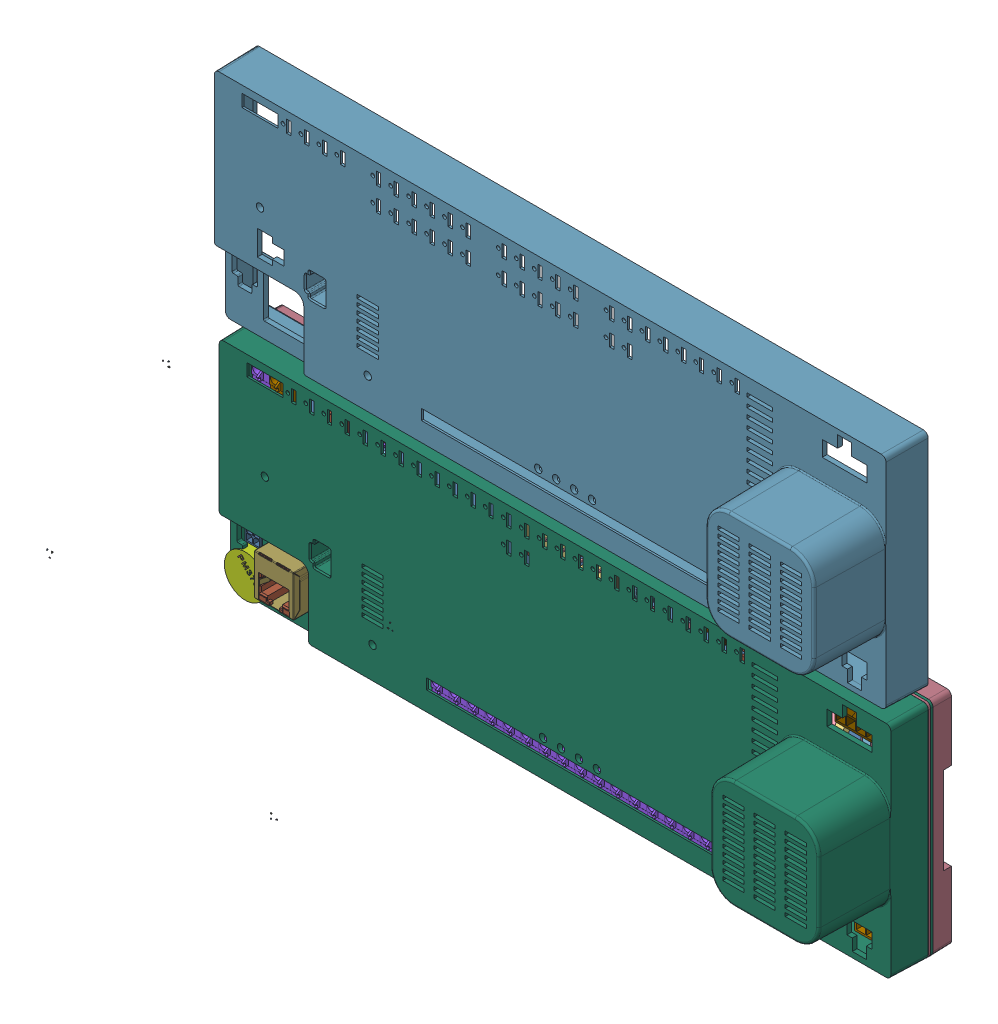
SolidWorks assembly _SC944D, configuration Default. Lengths in mm. (continued)
Components (placement in the parent): (continued)
- U10-1: U10 [Default] at origin size (22 22 1.6) (continued)
  - User_Library-LQFP144-1: User_Library-LQFP144 [Default] at (60.232 23.8429 0) x (-1 0 0) z (0 1 0) size (22 1.6 22) (continued)
    - User_Library-LQFP144_Assu_Fuss_LQFP144-4: User_Library-LQFP144_Assu_Fuss_LQFP144 [Default] at (-10 0 0) x (-1 0 0) z (0 0 -1) size (1 0.89 17.72) (continued)
      - User_Library-LQFP144_Fuss_LQFP144-3: User_Library-LQFP144_Fuss_LQFP144 [Default] at (0 0 -3.75) size (1 0.89 0.22)
      - User_Library-LQFP144_Fuss_LQFP144-4: User_Library-LQFP144_Fuss_LQFP144 [Default] at (0 0 -0.25) size (1 0.89 0.22)
      - User_Library-LQFP144_Fuss_LQFP144-5: User_Library-LQFP144_Fuss_LQFP144 [Default] at (0 0 -5.25) size (1 0.89 0.22)
      - User_Library-LQFP144_Fuss_LQFP144-6: User_Library-LQFP144_Fuss_LQFP144 [Default] at (0 0 -8.25) size (1 0.89 0.22)
      - User_Library-LQFP144_Fuss_LQFP144-7: User_Library-LQFP144_Fuss_LQFP144 [Default] at (0 0 -0.25) size (1 0.89 0.22)
      - User_Library-LQFP144_Fuss_LQFP144-8: User_Library-LQFP144_Fuss_LQFP144 [Default] at (0 0 -3.75) size (1 0.89 0.22)
      - User_Library-LQFP144_Fuss_LQFP144-9: User_Library-LQFP144_Fuss_LQFP144 [Default] at (0 0 -0.25) size (1 0.89 0.22)
      - User_Library-LQFP144_Fuss_LQFP144-10: User_Library-LQFP144_Fuss_LQFP144 [Default] at (0 0 6.75) size (1 0.89 0.22)
      - User_Library-LQFP144_Fuss_LQFP144-11: User_Library-LQFP144_Fuss_LQFP144 [Default] at (0 0 -3.75) size (1 0.89 0.22)
      - User_Library-LQFP144_Fuss_LQFP144-12: User_Library-LQFP144_Fuss_LQFP144 [Default] at (0 0 4.25) size (1 0.89 0.22)
      - User_Library-LQFP144_Fuss_LQFP144-13: User_Library-LQFP144_Fuss_LQFP144 [Default] at (0 0 0.75) size (1 0.89 0.22)
      - User_Library-LQFP144_Fuss_LQFP144-14: User_Library-LQFP144_Fuss_LQFP144 [Default] at (0 0 7.75) size (1 0.89 0.22)
      - User_Library-LQFP144_Fuss_LQFP144-15: User_Library-LQFP144_Fuss_LQFP144 [Default] at (0 0 1.75) size (1 0.89 0.22)
      - User_Library-LQFP144_Fuss_LQFP144-16: User_Library-LQFP144_Fuss_LQFP144 [Default] at (0 0 -2.25) size (1 0.89 0.22)
      - User_Library-LQFP144_Fuss_LQFP144-17: User_Library-LQFP144_Fuss_LQFP144 [Default] at (0 0 -2.75) size (1 0.89 0.22)
      - User_Library-LQFP144_Fuss_LQFP144-18: User_Library-LQFP144_Fuss_LQFP144 [Default] at (0 0 -4.25) size (1 0.89 0.22)
      - User_Library-LQFP144_Fuss_LQFP144-19: User_Library-LQFP144_Fuss_LQFP144 [Default] at (0 0 3.25) size (1 0.89 0.22)
      - User_Library-LQFP144_Fuss_LQFP144-20: User_Library-LQFP144_Fuss_LQFP144 [Default] at (0 0 -1.75) size (1 0.89 0.22)
      - User_Library-LQFP144_Fuss_LQFP144-21: User_Library-LQFP144_Fuss_LQFP144 [Default] at (0 0 -1.75) size (1 0.89 0.22)
      - User_Library-LQFP144_Fuss_LQFP144-22: User_Library-LQFP144_Fuss_LQFP144 [Default] at (0 0 2.75) size (1 0.89 0.22)
      - User_Library-LQFP144_Fuss_LQFP144-23: User_Library-LQFP144_Fuss_LQFP144 [Default] at (0 0 -2.75) size (1 0.89 0.22)
      - User_Library-LQFP144_Fuss_LQFP144-24: User_Library-LQFP144_Fuss_LQFP144 [Default] at (0 0 -3.75) size (1 0.89 0.22)
      - User_Library-LQFP144_Fuss_LQFP144-25: User_Library-LQFP144_Fuss_LQFP144 [Default] at (0 0 -5.75) size (1 0.89 0.22)
      - User_Library-LQFP144_Fuss_LQFP144-26: User_Library-LQFP144_Fuss_LQFP144 [Default] at (0 0 0.75) size (1 0.89 0.22)
      - User_Library-LQFP144_Fuss_LQFP144-27: User_Library-LQFP144_Fuss_LQFP144 [Default] at (0 0 -6.25) size (1 0.89 0.22)
      - User_Library-LQFP144_Fuss_LQFP144-28: User_Library-LQFP144_Fuss_LQFP144 [Default] at (0 0 -2.75) size (1 0.89 0.22)
      - User_Library-LQFP144_Fuss_LQFP144-29: User_Library-LQFP144_Fuss_LQFP144 [Default] at (0 0 1.25) size (1 0.89 0.22)
      - User_Library-LQFP144_Fuss_LQFP144-30: User_Library-LQFP144_Fuss_LQFP144 [Default] at (0 0 -0.25) size (1 0.89 0.22)
      - User_Library-LQFP144_Fuss_LQFP144-31: User_Library-LQFP144_Fuss_LQFP144 [Default] at (0 0 -1.25) size (1 0.89 0.22)
      - User_Library-LQFP144_Fuss_LQFP144-32: User_Library-LQFP144_Fuss_LQFP144 [Default] at (0 0 5.25) size (1 0.89 0.22)
      - User_Library-LQFP144_Fuss_LQFP144-33: User_Library-LQFP144_Fuss_LQFP144 [Default] at (0 0 8.25) size (1 0.89 0.22)
      - User_Library-LQFP144_Fuss_LQFP144-34: User_Library-LQFP144_Fuss_LQFP144 [Default] at (0 0 -6.25) size (1 0.89 0.22)
      - User_Library-LQFP144_Fuss_LQFP144-35: User_Library-LQFP144_Fuss_LQFP144 [Default] at (0 0 -0.75) size (1 0.89 0.22)
      - User_Library-LQFP144_Fuss_LQFP144-36: User_Library-LQFP144_Fuss_LQFP144 [Default] at (0 0 -8.75) size (1 0.89 0.22)
      - User_Library-LQFP144_Fuss_LQFP144-37: User_Library-LQFP144_Fuss_LQFP144 [Default] at (0 0 -1.25) size (1 0.89 0.22)
      - User_Library-LQFP144_Fuss_LQFP144-38: User_Library-LQFP144_Fuss_LQFP144 [Default] at (0 0 -1.25) size (1 0.89 0.22)
      - User_Library-LQFP144_Fuss_LQFP144-39: User_Library-LQFP144_Fuss_LQFP144 [Default] at (0 0 -2.75) size (1 0.89 0.22)
      - User_Library-LQFP144_Fuss_LQFP144-40: User_Library-LQFP144_Fuss_LQFP144 [Default] at (0 0 -2.75) size (1 0.89 0.22)
      - User_Library-LQFP144_Fuss_LQFP144-41: User_Library-LQFP144_Fuss_LQFP144 [Default] at (0 0 2.25) size (1 0.89 0.22)
      - User_Library-LQFP144_Fuss_LQFP144-42: User_Library-LQFP144_Fuss_LQFP144 [Default] at (0 0 3.75) size (1 0.89 0.22)
      - User_Library-LQFP144_Fuss_LQFP144-43: User_Library-LQFP144_Fuss_LQFP144 [Default] at (0 0 0.75) size (1 0.89 0.22)
      - User_Library-LQFP144_Fuss_LQFP144-44: User_Library-LQFP144_Fuss_LQFP144 [Default] at (0 0 0.75) size (1 0.89 0.22)
      - User_Library-LQFP144_Fuss_LQFP144-45: User_Library-LQFP144_Fuss_LQFP144 [Default] at (0 0 1.25) size (1 0.89 0.22)
      - User_Library-LQFP144_Fuss_LQFP144-46: User_Library-LQFP144_Fuss_LQFP144 [Default] at (0 0 1.75) size (1 0.89 0.22)
      - User_Library-LQFP144_Fuss_LQFP144-47: User_Library-LQFP144_Fuss_LQFP144 [Default] at (0 0 3.25) size (1 0.89 0.22)
      - User_Library-LQFP144_Fuss_LQFP144-48: User_Library-LQFP144_Fuss_LQFP144 [Default] at (0 0 -3.25) size (1 0.89 0.22)
      - User_Library-LQFP144_Fuss_LQFP144-49: User_Library-LQFP144_Fuss_LQFP144 [Default] at (0 0 5.75) size (1 0.89 0.22)
      - User_Library-LQFP144_Fuss_LQFP144-50: User_Library-LQFP144_Fuss_LQFP144 [Default] at (0 0 4.25) size (1 0.89 0.22)
      - User_Library-LQFP144_Fuss_LQFP144-51: User_Library-LQFP144_Fuss_LQFP144 [Default] at (0 0 3.25) size (1 0.89 0.22)
      - User_Library-LQFP144_Fuss_LQFP144-52: User_Library-LQFP144_Fuss_LQFP144 [Default] at (0 0 6.25) size (1 0.89 0.22)
      - User_Library-LQFP144_Fuss_LQFP144-53: User_Library-LQFP144_Fuss_LQFP144 [Default] at (0 0 -5.25) size (1 0.89 0.22)
      - User_Library-LQFP144_Fuss_LQFP144-54: User_Library-LQFP144_Fuss_LQFP144 [Default] at (0 0 -6.75) size (1 0.89 0.22)
      - User_Library-LQFP144_Fuss_LQFP144-55: User_Library-LQFP144_Fuss_LQFP144 [Default] at (0 0 -0.75) size (1 0.89 0.22)
      - User_Library-LQFP144_Fuss_LQFP144-56: User_Library-LQFP144_Fuss_LQFP144 [Default] at (0 0 1.75) size (1 0.89 0.22)
      - User_Library-LQFP144_Fuss_LQFP144-57: User_Library-LQFP144_Fuss_LQFP144 [Default] at (0 0 -3.25) size (1 0.89 0.22)
      - User_Library-LQFP144_Fuss_LQFP144-58: User_Library-LQFP144_Fuss_LQFP144 [Default] at (0 0 -4.25) size (1 0.89 0.22)
      - User_Library-LQFP144_Fuss_LQFP144-59: User_Library-LQFP144_Fuss_LQFP144 [Default] at (0 0 -5.25) size (1 0.89 0.22)
      - User_Library-LQFP144_Fuss_LQFP144-60: User_Library-LQFP144_Fuss_LQFP144 [Default] at (0 0 -1.25) size (1 0.89 0.22)
      - User_Library-LQFP144_Fuss_LQFP144-61: User_Library-LQFP144_Fuss_LQFP144 [Default] at (0 0 -0.75) size (1 0.89 0.22)
      - User_Library-LQFP144_Fuss_LQFP144-62: User_Library-LQFP144_Fuss_LQFP144 [Default] at (0 0 -6.25) size (1 0.89 0.22)
      - User_Library-LQFP144_Fuss_LQFP144-63: User_Library-LQFP144_Fuss_LQFP144 [Default] at (0 0 4.75) size (1 0.89 0.22)
      - User_Library-LQFP144_Fuss_LQFP144-64: User_Library-LQFP144_Fuss_LQFP144 [Default] at (0 0 3.25) size (1 0.89 0.22)
      - User_Library-LQFP144_Fuss_LQFP144-65: User_Library-LQFP144_Fuss_LQFP144 [Default] at (0 0 4.25) size (1 0.89 0.22)
      - User_Library-LQFP144_Fuss_LQFP144-66: User_Library-LQFP144_Fuss_LQFP144 [Default] at (0 0 0.25) size (1 0.89 0.22)
      - User_Library-LQFP144_Fuss_LQFP144-67: User_Library-LQFP144_Fuss_LQFP144 [Default] at (0 0 4.25) size (1 0.89 0.22)
      - User_Library-LQFP144_Fuss_LQFP144-68: User_Library-LQFP144_Fuss_LQFP144 [Default] at (0 0 6.75) size (1 0.89 0.22)
      - User_Library-LQFP144_Fuss_LQFP144-69: User_Library-LQFP144_Fuss_LQFP144 [Default] at (0 0 0.25) size (1 0.89 0.22)
      - User_Library-LQFP144_Fuss_LQFP144-70: User_Library-LQFP144_Fuss_LQFP144 [Default] at (0 0 0.25) size (1 0.89 0.22)
      - User_Library-LQFP144_Fuss_LQFP144-71: User_Library-LQFP144_Fuss_LQFP144 [Default] at (0 0 -1.25) size (1 0.89 0.22)
      - User_Library-LQFP144_Fuss_LQFP144-72: User_Library-LQFP144_Fuss_LQFP144 [Default] at (0 0 -3.75) size (1 0.89 0.22)
      - User_Library-LQFP144_Fuss_LQFP144-73: User_Library-LQFP144_Fuss_LQFP144 [Default] at (0 0 -0.25) size (1 0.89 0.22)
      - User_Library-LQFP144_Fuss_LQFP144-74: User_Library-LQFP144_Fuss_LQFP144 [Default] at (0 0 1.25) size (1 0.89 0.22)
      - User_Library-LQFP144_Fuss_LQFP144-75: User_Library-LQFP144_Fuss_LQFP144 [Default] at (0 0 0.75) size (1 0.89 0.22)
      - User_Library-LQFP144_Fuss_LQFP144-76: User_Library-LQFP144_Fuss_LQFP144 [Default] at (0 0 -7.75) size (1 0.89 0.22)
      - User_Library-LQFP144_Fuss_LQFP144-77: User_Library-LQFP144_Fuss_LQFP144 [Default] at (0 0 -3.25) size (1 0.89 0.22)
      - User_Library-LQFP144_Fuss_LQFP144-78: User_Library-LQFP144_Fuss_LQFP144 [Default] at (0 0 2.75) size (1 0.89 0.22)
      - User_Library-LQFP144_Fuss_LQFP144-79: User_Library-LQFP144_Fuss_LQFP144 [Default] at (0 0 4.75) size (1 0.89 0.22)
      - User_Library-LQFP144_Fuss_LQFP144-80: User_Library-LQFP144_Fuss_LQFP144 [Default] at (0 0 -7.25) size (1 0.89 0.22)
      - User_Library-LQFP144_Fuss_LQFP144-81: User_Library-LQFP144_Fuss_LQFP144 [Default] at (0 0 0.75) size (1 0.89 0.22)
      - User_Library-LQFP144_Fuss_LQFP144-82: User_Library-LQFP144_Fuss_LQFP144 [Default] at (0 0 0.75) size (1 0.89 0.22)
      - User_Library-LQFP144_Fuss_LQFP144-83: User_Library-LQFP144_Fuss_LQFP144 [Default] at (0 0 -0.75) size (1 0.89 0.22)
      - User_Library-LQFP144_Fuss_LQFP144-84: User_Library-LQFP144_Fuss_LQFP144 [Default] at (0 0 6.75) size (1 0.89 0.22)
      - User_Library-LQFP144_Fuss_LQFP144-85: User_Library-LQFP144_Fuss_LQFP144 [Default] at (0 0 -3.25) size (1 0.89 0.22)
      - User_Library-LQFP144_Fuss_LQFP144-86: User_Library-LQFP144_Fuss_LQFP144 [Default] at (0 0 3.75) size (1 0.89 0.22)
      - User_Library-LQFP144_Fuss_LQFP144-87: User_Library-LQFP144_Fuss_LQFP144 [Default] at (0 0 -0.75) size (1 0.89 0.22)
      - User_Library-LQFP144_Fuss_LQFP144-88: User_Library-LQFP144_Fuss_LQFP144 [Default] at (0 0 -1.75) size (1 0.89 0.22)
      - User_Library-LQFP144_Fuss_LQFP144-89: User_Library-LQFP144_Fuss_LQFP144 [Default] at (0 0 7.25) size (1 0.89 0.22)
      - User_Library-LQFP144_Fuss_LQFP144-90: User_Library-LQFP144_Fuss_LQFP144 [Default] at (0 0 0.75) size (1 0.89 0.22)
      - User_Library-LQFP144_Fuss_LQFP144-91: User_Library-LQFP144_Fuss_LQFP144 [Default] at (0 0 0.25) size (1 0.89 0.22)
      - User_Library-LQFP144_Fuss_LQFP144-92: User_Library-LQFP144_Fuss_LQFP144 [Default] at (0 0 0.25) size (1 0.89 0.22)
      - User_Library-LQFP144_Fuss_LQFP144-93: User_Library-LQFP144_Fuss_LQFP144 [Default] at (0 0 0.25) size (1 0.89 0.22)
      - User_Library-LQFP144_Fuss_LQFP144-94: User_Library-LQFP144_Fuss_LQFP144 [Default] at (0 0 1.75) size (1 0.89 0.22)
      - User_Library-LQFP144_Fuss_LQFP144-95: User_Library-LQFP144_Fuss_LQFP144 [Default] at (0 0 3.25) size (1 0.89 0.22)
      - User_Library-LQFP144_Fuss_LQFP144-96: User_Library-LQFP144_Fuss_LQFP144 [Default] at (0 0 -2.75) size (1 0.89 0.22)
      - User_Library-LQFP144_Fuss_LQFP144-97: User_Library-LQFP144_Fuss_LQFP144 [Default] at (0 0 -1.75) size (1 0.89 0.22)
      - User_Library-LQFP144_Fuss_LQFP144-98: User_Library-LQFP144_Fuss_LQFP144 [Default] at (0 0 4.75) size (1 0.89 0.22)
      - User_Library-LQFP144_Fuss_LQFP144-99: User_Library-LQFP144_Fuss_LQFP144 [Default] at (0 0 1.25) size (1 0.89 0.22)
      - User_Library-LQFP144_Fuss_LQFP144-100: User_Library-LQFP144_Fuss_LQFP144 [Default] at (0 0 4.75) size (1 0.89 0.22)
      - User_Library-LQFP144_Fuss_LQFP144-101: User_Library-LQFP144_Fuss_LQFP144 [Default] at (0 0 2.25) size (1 0.89 0.22)
      - User_Library-LQFP144_Fuss_LQFP144-102: User_Library-LQFP144_Fuss_LQFP144 [Default] at (0 0 2.25) size (1 0.89 0.22)
      - User_Library-LQFP144_Fuss_LQFP144-103: User_Library-LQFP144_Fuss_LQFP144 [Default] at (0 0 -2.75) size (1 0.89 0.22)
      - User_Library-LQFP144_Fuss_LQFP144-104: User_Library-LQFP144_Fuss_LQFP144 [Default] at (0 0 1.75) size (1 0.89 0.22)
      - User_Library-LQFP144_Fuss_LQFP144-105: User_Library-LQFP144_Fuss_LQFP144 [Default] at (0 0 7.25) size (1 0.89 0.22)
      - User_Library-LQFP144_Fuss_LQFP144-106: User_Library-LQFP144_Fuss_LQFP144 [Default] at (0 0 4.25) size (1 0.89 0.22)
      - User_Library-LQFP144_Fuss_LQFP144-107: User_Library-LQFP144_Fuss_LQFP144 [Default] at (0 0 7.75) size (1 0.89 0.22)
      - User_Library-LQFP144_Fuss_LQFP144-108: User_Library-LQFP144_Fuss_LQFP144 [Default] at (0 0 4.25) size (1 0.89 0.22)
      - User_Library-LQFP144_Fuss_LQFP144-109: User_Library-LQFP144_Fuss_LQFP144 [Default] at (0 0 7.25) size (1 0.89 0.22)
      - User_Library-LQFP144_Fuss_LQFP144-110: User_Library-LQFP144_Fuss_LQFP144 [Default] at (0 0 1.25) size (1 0.89 0.22)
      - User_Library-LQFP144_Fuss_LQFP144-111: User_Library-LQFP144_Fuss_LQFP144 [Default] at (0 0 7.25) size (1 0.89 0.22)
      - User_Library-LQFP144_Fuss_LQFP144-112: User_Library-LQFP144_Fuss_LQFP144 [Default] at (0 0 5.25) size (1 0.89 0.22)
      - User_Library-LQFP144_Fuss_LQFP144-113: User_Library-LQFP144_Fuss_LQFP144 [Default] at (0 0 6.75) size (1 0.89 0.22)
      - User_Library-LQFP144_Fuss_LQFP144-114: User_Library-LQFP144_Fuss_LQFP144 [Default] at (0 0 -6.25) size (1 0.89 0.22)
      - User_Library-LQFP144_Fuss_LQFP144-115: User_Library-LQFP144_Fuss_LQFP144 [Default] at (0 0 -0.25) size (1 0.89 0.22)
      - User_Library-LQFP144_Fuss_LQFP144-116: User_Library-LQFP144_Fuss_LQFP144 [Default] at (0 0 0.25) size (1 0.89 0.22)
      - User_Library-LQFP144_Fuss_LQFP144-117: User_Library-LQFP144_Fuss_LQFP144 [Default] at (0 0 8.25) size (1 0.89 0.22)
      - User_Library-LQFP144_Fuss_LQFP144-118: User_Library-LQFP144_Fuss_LQFP144 [Default] at (0 0 -4.75) size (1 0.89 0.22)
      - User_Library-LQFP144_Fuss_LQFP144-119: User_Library-LQFP144_Fuss_LQFP144 [Default] at (0 0 -2.25) size (1 0.89 0.22)
      - User_Library-LQFP144_Fuss_LQFP144-120: User_Library-LQFP144_Fuss_LQFP144 [Default] at (0 0 -6.75) size (1 0.89 0.22)
      - User_Library-LQFP144_Fuss_LQFP144-121: User_Library-LQFP144_Fuss_LQFP144 [Default] at (0 0 -1.75) size (1 0.89 0.22)
      - User_Library-LQFP144_Fuss_LQFP144-122: User_Library-LQFP144_Fuss_LQFP144 [Default] at (0 0 -7.25) size (1 0.89 0.22)
      - User_Library-LQFP144_Fuss_LQFP144-123: User_Library-LQFP144_Fuss_LQFP144 [Default] at (0 0 -5.25) size (1 0.89 0.22)
      - User_Library-LQFP144_Fuss_LQFP144-124: User_Library-LQFP144_Fuss_LQFP144 [Default] at (0 0 -5.75) size (1 0.89 0.22)
      - User_Library-LQFP144_Fuss_LQFP144-125: User_Library-LQFP144_Fuss_LQFP144 [Default] at (0 0 2.75) size (1 0.89 0.22)
      - User_Library-LQFP144_Fuss_LQFP144-126: User_Library-LQFP144_Fuss_LQFP144 [Default] at (0 0 1.75) size (1 0.89 0.22)
      - User_Library-LQFP144_Fuss_LQFP144-127: User_Library-LQFP144_Fuss_LQFP144 [Default] at (0 0 0.25) size (1 0.89 0.22)
      - User_Library-LQFP144_Fuss_LQFP144-128: User_Library-LQFP144_Fuss_LQFP144 [Default] at (0 0 -3.25) size (1 0.89 0.22)
      - User_Library-LQFP144_Fuss_LQFP144-129: User_Library-LQFP144_Fuss_LQFP144 [Default] at (0 0 3.25) size (1 0.89 0.22)
      - User_Library-LQFP144_Fuss_LQFP144-130: User_Library-LQFP144_Fuss_LQFP144 [Default] at (0 0 -2.75) size (1 0.89 0.22)
      - User_Library-LQFP144_Fuss_LQFP144-131: User_Library-LQFP144_Fuss_LQFP144 [Default] at (0 0 3.75) size (1 0.89 0.22)
      - User_Library-LQFP144_Fuss_LQFP144-132: User_Library-LQFP144_Fuss_LQFP144 [Default] at (0 0 0.25) size (1 0.89 0.22)
      - User_Library-LQFP144_Fuss_LQFP144-133: User_Library-LQFP144_Fuss_LQFP144 [Default] at (0 0 2.25) size (1 0.89 0.22)
      - User_Library-LQFP144_Fuss_LQFP144-134: User_Library-LQFP144_Fuss_LQFP144 [Default] at (0 0 -1.25) size (1 0.89 0.22)
      - User_Library-LQFP144_Fuss_LQFP144-135: User_Library-LQFP144_Fuss_LQFP144 [Default] at (0 0 -0.75) size (1 0.89 0.22)
      - User_Library-LQFP144_Fuss_LQFP144-136: User_Library-LQFP144_Fuss_LQFP144 [Default] at (0 0 -4.25) size (1 0.89 0.22)
      - User_Library-LQFP144_Fuss_LQFP144-137: User_Library-LQFP144_Fuss_LQFP144 [Default] at (0 0 1.75) size (1 0.89 0.22)
      - User_Library-LQFP144_Fuss_LQFP144-138: User_Library-LQFP144_Fuss_LQFP144 [Default] at (0 0 -1.25) size (1 0.89 0.22)
      - User_Library-LQFP144_Fuss_LQFP144-139: User_Library-LQFP144_Fuss_LQFP144 [Default] at (0 0 -1.75) size (1 0.89 0.22)
      - User_Library-LQFP144_Fuss_LQFP144-140: User_Library-LQFP144_Fuss_LQFP144 [Default] at (0 0 4.25) size (1 0.89 0.22)
      - User_Library-LQFP144_Fuss_LQFP144-141: User_Library-LQFP144_Fuss_LQFP144 [Default] at (0 0 -2.25) size (1 0.89 0.22)
      - User_Library-LQFP144_Fuss_LQFP144-142: User_Library-LQFP144_Fuss_LQFP144 [Default] at (0 0 5.25) size (1 0.89 0.22)
      - User_Library-LQFP144_Fuss_LQFP144-143: User_Library-LQFP144_Fuss_LQFP144 [Default] at (0 0 2.75) size (1 0.89 0.22)
      - User_Library-LQFP144_Fuss_LQFP144-144: User_Library-LQFP144_Fuss_LQFP144 [Default] at (0 0 -1.75) size (1 0.89 0.22)
      - User_Library-LQFP144_Fuss_LQFP144-145: User_Library-LQFP144_Fuss_LQFP144 [Default] at (0 0 -0.25) size (1 0.89 0.22)
      - User_Library-LQFP144_Fuss_LQFP144-146: User_Library-LQFP144_Fuss_LQFP144 [Default] at (0 0 0.75) size (1 0.89 0.22)
      - User_Library-LQFP144_Fuss_LQFP144-147: User_Library-LQFP144_Fuss_LQFP144 [Default] at (0 0 -0.25) size (1 0.89 0.22)
      - User_Library-LQFP144_Fuss_LQFP144-148: User_Library-LQFP144_Fuss_LQFP144 [Default] at (0 0 3.75) size (1 0.89 0.22)
      - User_Library-LQFP144_Fuss_LQFP144-149: User_Library-LQFP144_Fuss_LQFP144 [Default] at (0 0 2.75) size (1 0.89 0.22)
      - User_Library-LQFP144_Fuss_LQFP144-150: User_Library-LQFP144_Fuss_LQFP144 [Default] at (0 0 2.75) size (1 0.89 0.22)
      - User_Library-LQFP144_Fuss_LQFP144-151: User_Library-LQFP144_Fuss_LQFP144 [Default] at (0 0 6.25) size (1 0.89 0.22)
      - User_Library-LQFP144_Fuss_LQFP144-152: User_Library-LQFP144_Fuss_LQFP144 [Default] at (0 0 2.25) size (1 0.89 0.22)
      - User_Library-LQFP144_Fuss_LQFP144-153: User_Library-LQFP144_Fuss_LQFP144 [Default] at (0 0 -0.75) size (1 0.89 0.22)
      - User_Library-LQFP144_Fuss_LQFP144-154: User_Library-LQFP144_Fuss_LQFP144 [Default] at (0 0 -2.25) size (1 0.89 0.22)
      - User_Library-LQFP144_Fuss_LQFP144-155: User_Library-LQFP144_Fuss_LQFP144 [Default] at (0 0 -0.75) size (1 0.89 0.22)
      - User_Library-LQFP144_Fuss_LQFP144-156: User_Library-LQFP144_Fuss_LQFP144 [Default] at (0 0 -2.25) size (1 0.89 0.22)
      - User_Library-LQFP144_Fuss_LQFP144-157: User_Library-LQFP144_Fuss_LQFP144 [Default] at (0 0 -2.25) size (1 0.89 0.22)
      - User_Library-LQFP144_Fuss_LQFP144-158: User_Library-LQFP144_Fuss_LQFP144 [Default] at (0 0 0.75) size (1 0.89 0.22)
      - User_Library-LQFP144_Fuss_LQFP144-159: User_Library-LQFP144_Fuss_LQFP144 [Default] at (0 0 -4.25) size (1 0.89 0.22)
      - User_Library-LQFP144_Fuss_LQFP144-160: User_Library-LQFP144_Fuss_LQFP144 [Default] at (0 0 4.25) size (1 0.89 0.22)
      - User_Library-LQFP144_Fuss_LQFP144-161: User_Library-LQFP144_Fuss_LQFP144 [Default] at (0 0 1.25) size (1 0.89 0.22)
      - User_Library-LQFP144_Fuss_LQFP144-162: User_Library-LQFP144_Fuss_LQFP144 [Default] at (0 0 -0.25) size (1 0.89 0.22)
      - User_Library-LQFP144_Fuss_LQFP144-163: User_Library-LQFP144_Fuss_LQFP144 [Default] at (0 0 -4.25) size (1 0.89 0.22)
      - User_Library-LQFP144_Fuss_LQFP144-164: User_Library-LQFP144_Fuss_LQFP144 [Default] at (0 0 -1.25) size (1 0.89 0.22)
      - User_Library-LQFP144_Fuss_LQFP144-165: User_Library-LQFP144_Fuss_LQFP144 [Default] at (0 0 -8.25) size (1 0.89 0.22)
      - User_Library-LQFP144_Fuss_LQFP144-166: User_Library-LQFP144_Fuss_LQFP144 [Default] at (0 0 -3.25) size (1 0.89 0.22)
      - User_Library-LQFP144_Fuss_LQFP144-167: User_Library-LQFP144_Fuss_LQFP144 [Default] at (0 0 -4.75) size (1 0.89 0.22)
      - User_Library-LQFP144_Fuss_LQFP144-168: User_Library-LQFP144_Fuss_LQFP144 [Default] at (0 0 -2.25) size (1 0.89 0.22)
      - User_Library-LQFP144_Fuss_LQFP144-169: User_Library-LQFP144_Fuss_LQFP144 [Default] at (0 0 -1.25) size (1 0.89 0.22)
      - User_Library-LQFP144_Fuss_LQFP144-170: User_Library-LQFP144_Fuss_LQFP144 [Default] at (0 0 -7.25) size (1 0.89 0.22)
      - User_Library-LQFP144_Fuss_LQFP144-171: User_Library-LQFP144_Fuss_LQFP144 [Default] at (0 0 -4.25) size (1 0.89 0.22)
      - User_Library-LQFP144_Fuss_LQFP144-172: User_Library-LQFP144_Fuss_LQFP144 [Default] at (0 0 -4.25) size (1 0.89 0.22)
      - User_Library-LQFP144_Fuss_LQFP144-173: User_Library-LQFP144_Fuss_LQFP144 [Default] at (0 0 1.75) size (1 0.89 0.22)
      - User_Library-LQFP144_Fuss_LQFP144-174: User_Library-LQFP144_Fuss_LQFP144 [Default] at (0 0 0.25) size (1 0.89 0.22)
      - User_Library-LQFP144_Fuss_LQFP144-175: User_Library-LQFP144_Fuss_LQFP144 [Default] at (0 0 -0.75) size (1 0.89 0.22)
      - User_Library-LQFP144_Fuss_LQFP144-176: User_Library-LQFP144_Fuss_LQFP144 [Default] at (0 0 0.75) size (1 0.89 0.22)
      - User_Library-LQFP144_Fuss_LQFP144-177: User_Library-LQFP144_Fuss_LQFP144 [Default] at (0 0 1.75) size (1 0.89 0.22)
      - User_Library-LQFP144_Fuss_LQFP144-178: User_Library-LQFP144_Fuss_LQFP144 [Default] at (0 0 -0.75) size (1 0.89 0.22)
      - User_Library-LQFP144_Fuss_LQFP144-179: User_Library-LQFP144_Fuss_LQFP144 [Default] at (0 0 3.75) size (1 0.89 0.22)
      - User_Library-LQFP144_Fuss_LQFP144-180: User_Library-LQFP144_Fuss_LQFP144 [Default] at (0 0 4.75) size (1 0.89 0.22)
      - User_Library-LQFP144_Fuss_LQFP144-181: User_Library-LQFP144_Fuss_LQFP144 [Default] at (0 0 -0.75) size (1 0.89 0.22)
      - User_Library-LQFP144_Fuss_LQFP144-182: User_Library-LQFP144_Fuss_LQFP144 [Default] at (0 0 2.75) size (1 0.89 0.22)
      - User_Library-LQFP144_Fuss_LQFP144-183: User_Library-LQFP144_Fuss_LQFP144 [Default] at (0 0 -1.25) size (1 0.89 0.22)
      - User_Library-LQFP144_Fuss_LQFP144-184: User_Library-LQFP144_Fuss_LQFP144 [Default] at (0 0 2.75) size (1 0.89 0.22)
      - User_Library-LQFP144_Fuss_LQFP144-185: User_Library-LQFP144_Fuss_LQFP144 [Default] at (0 0 5.25) size (1 0.89 0.22)
      - User_Library-LQFP144_Fuss_LQFP144-186: User_Library-LQFP144_Fuss_LQFP144 [Default] at (0 0 -4.25) size (1 0.89 0.22)
      - User_Library-LQFP144_Fuss_LQFP144-187: User_Library-LQFP144_Fuss_LQFP144 [Default] at (0 0 -4.75) size (1 0.89 0.22)
      - User_Library-LQFP144_Fuss_LQFP144-188: User_Library-LQFP144_Fuss_LQFP144 [Default] at (0 0 -3.75) size (1 0.89 0.22)
      - User_Library-LQFP144_Fuss_LQFP144-189: User_Library-LQFP144_Fuss_LQFP144 [Default] at (0 0 -6.25) size (1 0.89 0.22)
      - User_Library-LQFP144_Fuss_LQFP144-190: User_Library-LQFP144_Fuss_LQFP144 [Default] at (0 0 0.75) size (1 0.89 0.22)
      - User_Library-LQFP144_Fuss_LQFP144-191: User_Library-LQFP144_Fuss_LQFP144 [Default] at (0 0 0.25) size (1 0.89 0.22)
      - User_Library-LQFP144_Fuss_LQFP144-192: User_Library-LQFP144_Fuss_LQFP144 [Default] at (0 0 -0.25) size (1 0.89 0.22)
      - User_Library-LQFP144_Fuss_LQFP144-193: User_Library-LQFP144_Fuss_LQFP144 [Default] at (0 0 -3.25) size (1 0.89 0.22)
      - User_Library-LQFP144_Fuss_LQFP144-194: User_Library-LQFP144_Fuss_LQFP144 [Default] at (0 0 1.75) size (1 0.89 0.22)
      - User_Library-LQFP144_Fuss_LQFP144-195: User_Library-LQFP144_Fuss_LQFP144 [Default] at (0 0 0.25) size (1 0.89 0.22)
      - User_Library-LQFP144_Fuss_LQFP144-196: User_Library-LQFP144_Fuss_LQFP144 [Default] at (0 0 5.25) size (1 0.89 0.22)
      - User_Library-LQFP144_Fuss_LQFP144-197: User_Library-LQFP144_Fuss_LQFP144 [Default] at (0 0 -1.75) size (1 0.89 0.22)
      - User_Library-LQFP144_Fuss_LQFP144-198: User_Library-LQFP144_Fuss_LQFP144 [Default] at (0 0 5.75) size (1 0.89 0.22)
      - User_Library-LQFP144_Fuss_LQFP144-199: User_Library-LQFP144_Fuss_LQFP144 [Default] at (0 0 5.75) size (1 0.89 0.22)
      - User_Library-LQFP144_Fuss_LQFP144-200: User_Library-LQFP144_Fuss_LQFP144 [Default] at (0 0 3.25) size (1 0.89 0.22)
      - User_Library-LQFP144_Fuss_LQFP144-201: User_Library-LQFP144_Fuss_LQFP144 [Default] at (0 0 0.25) size (1 0.89 0.22)
      - User_Library-LQFP144_Fuss_LQFP144-202: User_Library-LQFP144_Fuss_LQFP144 [Default] at (0 0 -1.75) size (1 0.89 0.22)
      - User_Library-LQFP144_Fuss_LQFP144-203: User_Library-LQFP144_Fuss_LQFP144 [Default] at (0 0 -5.75) size (1 0.89 0.22)
      - User_Library-LQFP144_Fuss_LQFP144-204: User_Library-LQFP144_Fuss_LQFP144 [Default] at (0 0 1.25) size (1 0.89 0.22)
      - User_Library-LQFP144_Fuss_LQFP144-205: User_Library-LQFP144_Fuss_LQFP144 [Default] at (0 0 2.25) size (1 0.89 0.22)
      - User_Library-LQFP144_Fuss_LQFP144-206: User_Library-LQFP144_Fuss_LQFP144 [Default] at (0 0 -1.25) size (1 0.89 0.22)
      - User_Library-LQFP144_Fuss_LQFP144-207: User_Library-LQFP144_Fuss_LQFP144 [Default] at (0 0 -1.25) size (1 0.89 0.22)
      - User_Library-LQFP144_Fuss_LQFP144-208: User_Library-LQFP144_Fuss_LQFP144 [Default] at (0 0 -0.25) size (1 0.89 0.22)
      - User_Library-LQFP144_Fuss_LQFP144-209: User_Library-LQFP144_Fuss_LQFP144 [Default] at (0 0 1.25) size (1 0.89 0.22)
      - User_Library-LQFP144_Fuss_LQFP144-210: User_Library-LQFP144_Fuss_LQFP144 [Default] at (0 0 6.25) size (1 0.89 0.22)
      - User_Library-LQFP144_Fuss_LQFP144-211: User_Library-LQFP144_Fuss_LQFP144 [Default] at (0 0 5.75) size (1 0.89 0.22)
      - User_Library-LQFP144_Fuss_LQFP144-212: User_Library-LQFP144_Fuss_LQFP144 [Default] at (0 0 1.25) size (1 0.89 0.22)
      - User_Library-LQFP144_Fuss_LQFP144-213: User_Library-LQFP144_Fuss_LQFP144 [Default] at (0 0 -0.25) size (1 0.89 0.22)
      - User_Library-LQFP144_Fuss_LQFP144-214: User_Library-LQFP144_Fuss_LQFP144 [Default] at (0 0 6.25) size (1 0.89 0.22)
      - User_Library-LQFP144_Fuss_LQFP144-215: User_Library-LQFP144_Fuss_LQFP144 [Default] at (0 0 -0.75) size (1 0.89 0.22)
      - User_Library-LQFP144_Fuss_LQFP144-216: User_Library-LQFP144_Fuss_LQFP144 [Default] at (0 0 5.25) size (1 0.89 0.22)
      - User_Library-LQFP144_Fuss_LQFP144-217: User_Library-LQFP144_Fuss_LQFP144 [Default] at (0 0 -2.25) size (1 0.89 0.22)
      - User_Library-LQFP144_Fuss_LQFP144-218: User_Library-LQFP144_Fuss_LQFP144 [Default] at (0 0 2.75) size (1 0.89 0.22)
      - User_Library-LQFP144_Fuss_LQFP144-219: User_Library-LQFP144_Fuss_LQFP144 [Default] at (0 0 -1.75) size (1 0.89 0.22)
      - User_Library-LQFP144_Fuss_LQFP144-220: User_Library-LQFP144_Fuss_LQFP144 [Default] at (0 0 -5.25) size (1 0.89 0.22)
      - User_Library-LQFP144_Fuss_LQFP144-221: User_Library-LQFP144_Fuss_LQFP144 [Default] at (0 0 1.25) size (1 0.89 0.22)
      - User_Library-LQFP144_Fuss_LQFP144-222: User_Library-LQFP144_Fuss_LQFP144 [Default] at (0 0 -4.25) size (1 0.89 0.22)
      - User_Library-LQFP144_Fuss_LQFP144-223: User_Library-LQFP144_Fuss_LQFP144 [Default] at (0 0 -0.25) size (1 0.89 0.22)
      - User_Library-LQFP144_Fuss_LQFP144-224: User_Library-LQFP144_Fuss_LQFP144 [Default] at (0 0 2.75) size (1 0.89 0.22)
      - User_Library-LQFP144_Fuss_LQFP144-225: User_Library-LQFP144_Fuss_LQFP144 [Default] at (0 0 -0.75) size (1 0.89 0.22)
      - User_Library-LQFP144_Fuss_LQFP144-226: User_Library-LQFP144_Fuss_LQFP144 [Default] at (0 0 -1.75) size (1 0.89 0.22)
      - User_Library-LQFP144_Fuss_LQFP144-227: User_Library-LQFP144_Fuss_LQFP144 [Default] at (0 0 -7.25) size (1 0.89 0.22)
      - User_Library-LQFP144_Fuss_LQFP144-228: User_Library-LQFP144_Fuss_LQFP144 [Default] at (0 0 -6.75) size (1 0.89 0.22)
      - User_Library-LQFP144_Fuss_LQFP144-229: User_Library-LQFP144_Fuss_LQFP144 [Default] at (0 0 -0.25) size (1 0.89 0.22)
      - User_Library-LQFP144_Fuss_LQFP144-230: User_Library-LQFP144_Fuss_LQFP144 [Default] at (0 0 -2.25) size (1 0.89 0.22)
      - User_Library-LQFP144_Fuss_LQFP144-231: User_Library-LQFP144_Fuss_LQFP144 [Default] at (0 0 -3.75) size (1 0.89 0.22)
      - User_Library-LQFP144_Fuss_LQFP144-232: User_Library-LQFP144_Fuss_LQFP144 [Default] at (0 0 -4.75) size (1 0.89 0.22)
      - User_Library-LQFP144_Fuss_LQFP144-233: User_Library-LQFP144_Fuss_LQFP144 [Default] at (0 0 1.75) size (1 0.89 0.22)
      - User_Library-LQFP144_Fuss_LQFP144-234: User_Library-LQFP144_Fuss_LQFP144 [Default] at (0 0 -1.25) size (1 0.89 0.22)
      - User_Library-LQFP144_Fuss_LQFP144-235: User_Library-LQFP144_Fuss_LQFP144 [Default] at (0 0 8.75) size (1 0.89 0.22)
      - User_Library-LQFP144_Fuss_LQFP144-236: User_Library-LQFP144_Fuss_LQFP144 [Default] at (0 0 -0.75) size (1 0.89 0.22)
      - User_Library-LQFP144_Fuss_LQFP144-237: User_Library-LQFP144_Fuss_LQFP144 [Default] at (0 0 3.25) size (1 0.89 0.22)
      - User_Library-LQFP144_Fuss_LQFP144-238: User_Library-LQFP144_Fuss_LQFP144 [Default] at (0 0 6.75) size (1 0.89 0.22)
      - User_Library-LQFP144_Fuss_LQFP144-239: User_Library-LQFP144_Fuss_LQFP144 [Default] at (0 0 2.25) size (1 0.89 0.22)
      - User_Library-LQFP144_Fuss_LQFP144-240: User_Library-LQFP144_Fuss_LQFP144 [Default] at (0 0 -2.75) size (1 0.89 0.22)
      - User_Library-LQFP144_Fuss_LQFP144-241: User_Library-LQFP144_Fuss_LQFP144 [Default] at (0 0 -3.75) size (1 0.89 0.22)
      - User_Library-LQFP144_Fuss_LQFP144-242: User_Library-LQFP144_Fuss_LQFP144 [Default] at (0 0 4.75) size (1 0.89 0.22)
      - User_Library-LQFP144_Fuss_LQFP144-243: User_Library-LQFP144_Fuss_LQFP144 [Default] at (0 0 -0.25) size (1 0.89 0.22)
      - User_Library-LQFP144_Fuss_LQFP144-244: User_Library-LQFP144_Fuss_LQFP144 [Default] at (0 0 3.75) size (1 0.89 0.22)
      - User_Library-LQFP144_Fuss_LQFP144-245: User_Library-LQFP144_Fuss_LQFP144 [Default] at (0 0 -4.25) size (1 0.89 0.22)
      - User_Library-LQFP144_Fuss_LQFP144-246: User_Library-LQFP144_Fuss_LQFP144 [Default] at (0 0 -5.25) size (1 0.89 0.22)
      - User_Library-LQFP144_Fuss_LQFP144-247: User_Library-LQFP144_Fuss_LQFP144 [Default] at (0 0 -4.75) size (1 0.89 0.22)
      - User_Library-LQFP144_Fuss_LQFP144-248: User_Library-LQFP144_Fuss_LQFP144 [Default] at (0 0 -4.75) size (1 0.89 0.22)
      - User_Library-LQFP144_Fuss_LQFP144-249: User_Library-LQFP144_Fuss_LQFP144 [Default] at (0 0 -2.75) size (1 0.89 0.22)
      - User_Library-LQFP144_Fuss_LQFP144-250: User_Library-LQFP144_Fuss_LQFP144 [Default] at (0 0 -3.25) size (1 0.89 0.22)
      - User_Library-LQFP144_Fuss_LQFP144-251: User_Library-LQFP144_Fuss_LQFP144 [Default] at (0 0 0.25) size (1 0.89 0.22)
      - User_Library-LQFP144_Fuss_LQFP144-252: User_Library-LQFP144_Fuss_LQFP144 [Default] at (0 0 -6.75) size (1 0.89 0.22)
      - User_Library-LQFP144_Fuss_LQFP144-253: User_Library-LQFP144_Fuss_LQFP144 [Default] at (0 0 -7.75) size (1 0.89 0.22)
      - User_Library-LQFP144_Fuss_LQFP144-254: User_Library-LQFP144_Fuss_LQFP144 [Default] at (0 0 1.25) size (1 0.89 0.22)
      - User_Library-LQFP144_Fuss_LQFP144-255: User_Library-LQFP144_Fuss_LQFP144 [Default] at (0 0 2.25) size (1 0.89 0.22)
      - User_Library-LQFP144_Fuss_LQFP144-256: User_Library-LQFP144_Fuss_LQFP144 [Default] at (0 0 5.75) size (1 0.89 0.22)
      - User_Library-LQFP144_Fuss_LQFP144-257: User_Library-LQFP144_Fuss_LQFP144 [Default] at (0 0 2.25) size (1 0.89 0.22)
      - User_Library-LQFP144_Fuss_LQFP144-258: User_Library-LQFP144_Fuss_LQFP144 [Default] at (0 0 -0.75) size (1 0.89 0.22)
      - User_Library-LQFP144_Fuss_LQFP144-259: User_Library-LQFP144_Fuss_LQFP144 [Default] at (0 0 3.25) size (1 0.89 0.22)
      - User_Library-LQFP144_Fuss_LQFP144-260: User_Library-LQFP144_Fuss_LQFP144 [Default] at (0 0 -0.25) size (1 0.89 0.22)
      - User_Library-LQFP144_Fuss_LQFP144-261: User_Library-LQFP144_Fuss_LQFP144 [Default] at (0 0 -1.75) size (1 0.89 0.22)
      - User_Library-LQFP144_Fuss_LQFP144-262: User_Library-LQFP144_Fuss_LQFP144 [Default] at (0 0 -4.75) size (1 0.89 0.22)
      - User_Library-LQFP144_Fuss_LQFP144-263: User_Library-LQFP144_Fuss_LQFP144 [Default] at (0 0 0.75) size (1 0.89 0.22)
      - User_Library-LQFP144_Fuss_LQFP144-264: User_Library-LQFP144_Fuss_LQFP144 [Default] at (0 0 1.25) size (1 0.89 0.22)
      - User_Library-LQFP144_Fuss_LQFP144-265: User_Library-LQFP144_Fuss_LQFP144 [Default] at (0 0 -5.75) size (1 0.89 0.22)
      - User_Library-LQFP144_Fuss_LQFP144-266: User_Library-LQFP144_Fuss_LQFP144 [Default] at (0 0 -2.25) size (1 0.89 0.22)
      - User_Library-LQFP144_Fuss_LQFP144-267: User_Library-LQFP144_Fuss_LQFP144 [Default] at (0 0 -5.25) size (1 0.89 0.22)
      - User_Library-LQFP144_Fuss_LQFP144-268: User_Library-LQFP144_Fuss_LQFP144 [Default] at (0 0 -1.75) size (1 0.89 0.22)
      - User_Library-LQFP144_Fuss_LQFP144-269: User_Library-LQFP144_Fuss_LQFP144 [Default] at (0 0 0.75) size (1 0.89 0.22)
      - User_Library-LQFP144_Fuss_LQFP144-270: User_Library-LQFP144_Fuss_LQFP144 [Default] at (0 0 -1.25) size (1 0.89 0.22)
      - User_Library-LQFP144_Fuss_LQFP144-271: User_Library-LQFP144_Fuss_LQFP144 [Default] at (0 0 6.25) size (1 0.89 0.22)
      - User_Library-LQFP144_Fuss_LQFP144-272: User_Library-LQFP144_Fuss_LQFP144 [Default] at (0 0 3.75) size (1 0.89 0.22)
      - User_Library-LQFP144_Fuss_LQFP144-273: User_Library-LQFP144_Fuss_LQFP144 [Default] at (0 0 6.25) size (1 0.89 0.22)
      - User_Library-LQFP144_Fuss_LQFP144-274: User_Library-LQFP144_Fuss_LQFP144 [Default] at (0 0 0.25) size (1 0.89 0.22)
      - User_Library-LQFP144_Fuss_LQFP144-275: User_Library-LQFP144_Fuss_LQFP144 [Default] at (0 0 3.75) size (1 0.89 0.22)
      - User_Library-LQFP144_Fuss_LQFP144-276: User_Library-LQFP144_Fuss_LQFP144 [Default] at (0 0 1.75) size (1 0.89 0.22)
      - User_Library-LQFP144_Fuss_LQFP144-277: User_Library-LQFP144_Fuss_LQFP144 [Default] at (0 0 5.75) size (1 0.89 0.22)
      - User_Library-LQFP144_Fuss_LQFP144-278: User_Library-LQFP144_Fuss_LQFP144 [Default] at (0 0 -3.25) size (1 0.89 0.22)
      - User_Library-LQFP144_Fuss_LQFP144-279: User_Library-LQFP144_Fuss_LQFP144 [Default] at (0 0 -2.75) size (1 0.89 0.22)
      - User_Library-LQFP144_Fuss_LQFP144-280: User_Library-LQFP144_Fuss_LQFP144 [Default] at (0 0 -4.75) size (1 0.89 0.22)
      - User_Library-LQFP144_Fuss_LQFP144-281: User_Library-LQFP144_Fuss_LQFP144 [Default] at (0 0 -4.75) size (1 0.89 0.22)
      - User_Library-LQFP144_Fuss_LQFP144-282: User_Library-LQFP144_Fuss_LQFP144 [Default] at (0 0 0.25) size (1 0.89 0.22)
      - User_Library-LQFP144_Fuss_LQFP144-283: User_Library-LQFP144_Fuss_LQFP144 [Default] at (0 0 1.75) size (1 0.89 0.22)
      - User_Library-LQFP144_Fuss_LQFP144-284: User_Library-LQFP144_Fuss_LQFP144 [Default] at (0 0 -2.25) size (1 0.89 0.22)
      - User_Library-LQFP144_Fuss_LQFP144-285: User_Library-LQFP144_Fuss_LQFP144 [Default] at (0 0 -6.25) size (1 0.89 0.22)
      - User_Library-LQFP144_Fuss_LQFP144-286: User_Library-LQFP144_Fuss_LQFP144 [Default] at (0 0 -0.25) size (1 0.89 0.22)
      - User_Library-LQFP144_Fuss_LQFP144-287: User_Library-LQFP144_Fuss_LQFP144 [Default] at (0 0 1.75) size (1 0.89 0.22)
      - User_Library-LQFP144_Fuss_LQFP144-288: User_Library-LQFP144_Fuss_LQFP144 [Default] at (0 0 4.75) size (1 0.89 0.22)
      - User_Library-LQFP144_Fuss_LQFP144-289: User_Library-LQFP144_Fuss_LQFP144 [Default] at (0 0 -3.25) size (1 0.89 0.22)
      - User_Library-LQFP144_Fuss_LQFP144-290: User_Library-LQFP144_Fuss_LQFP144 [Default] at (0 0 7.75) size (1 0.89 0.22)
      - User_Library-LQFP144_Fuss_LQFP144-291: User_Library-LQFP144_Fuss_LQFP144 [Default] at (0 0 -7.75) size (1 0.89 0.22)
      - User_Library-LQFP144_Fuss_LQFP144-292: User_Library-LQFP144_Fuss_LQFP144 [Default] at (0 0 1.25) size (1 0.89 0.22)
      - User_Library-LQFP144_Fuss_LQFP144-293: User_Library-LQFP144_Fuss_LQFP144 [Default] at (0 0 5.25) size (1 0.89 0.22)
      - User_Library-LQFP144_Fuss_LQFP144-294: User_Library-LQFP144_Fuss_LQFP144 [Default] at (0 0 -0.75) size (1 0.89 0.22)
      - User_Library-LQFP144_Fuss_LQFP144-295: User_Library-LQFP144_Fuss_LQFP144 [Default] at (0 0 5.75) size (1 0.89 0.22)
      - User_Library-LQFP144_Fuss_LQFP144-296: User_Library-LQFP144_Fuss_LQFP144 [Default] at (0 0 2.75) size (1 0.89 0.22)
      - User_Library-LQFP144_Fuss_LQFP144-297: User_Library-LQFP144_Fuss_LQFP144 [Default] at (0 0 -1.75) size (1 0.89 0.22)
      - User_Library-LQFP144_Fuss_LQFP144-298: User_Library-LQFP144_Fuss_LQFP144 [Default] at (0 0 2.25) size (1 0.89 0.22)
      - User_Library-LQFP144_Fuss_LQFP144-299: User_Library-LQFP144_Fuss_LQFP144 [Default] at (0 0 1.25) size (1 0.89 0.22)
      - User_Library-LQFP144_Fuss_LQFP144-300: User_Library-LQFP144_Fuss_LQFP144 [Default] at (0 0 3.75) size (1 0.89 0.22)
      - User_Library-LQFP144_Fuss_LQFP144-301: User_Library-LQFP144_Fuss_LQFP144 [Default] at (0 0 -3.75) size (1 0.89 0.22)
      - User_Library-LQFP144_Fuss_LQFP144-302: User_Library-LQFP144_Fuss_LQFP144 [Default] at (0 0 0.75) size (1 0.89 0.22)
      - User_Library-LQFP144_Fuss_LQFP144-303: User_Library-LQFP144_Fuss_LQFP144 [Default] at (0 0 -6.75) size (1 0.89 0.22)
      - User_Library-LQFP144_Fuss_LQFP144-304: User_Library-LQFP144_Fuss_LQFP144 [Default] at (0 0 -3.25) size (1 0.89 0.22)
      - User_Library-LQFP144_Fuss_LQFP144-305: User_Library-LQFP144_Fuss_LQFP144 [Default] at (0 0 2.25) size (1 0.89 0.22)
      - User_Library-LQFP144_Fuss_LQFP144-306: User_Library-LQFP144_Fuss_LQFP144 [Default] at (0 0 -5.75) size (1 0.89 0.22)
      - User_Library-LQFP144_Fuss_LQFP144-307: User_Library-LQFP144_Fuss_LQFP144 [Default] at (0 0 0.25) size (1 0.89 0.22)
      - User_Library-LQFP144_Fuss_LQFP144-308: User_Library-LQFP144_Fuss_LQFP144 [Default] at (0 0 1.75) size (1 0.89 0.22)
      - User_Library-LQFP144_Fuss_LQFP144-309: User_Library-LQFP144_Fuss_LQFP144 [Default] at (0 0 -5.75) size (1 0.89 0.22)
      - User_Library-LQFP144_Fuss_LQFP144-310: User_Library-LQFP144_Fuss_LQFP144 [Default] at (0 0 -3.25) size (1 0.89 0.22)
      - User_Library-LQFP144_Fuss_LQFP144-311: User_Library-LQFP144_Fuss_LQFP144 [Default] at (0 0 -0.75) size (1 0.89 0.22)
      - User_Library-LQFP144_Fuss_LQFP144-312: User_Library-LQFP144_Fuss_LQFP144 [Default] at (0 0 -1.75) size (1 0.89 0.22)
      - User_Library-LQFP144_Fuss_LQFP144-313: User_Library-LQFP144_Fuss_LQFP144 [Default] at (0 0 2.25) size (1 0.89 0.22)
      - User_Library-LQFP144_Fuss_LQFP144-314: User_Library-LQFP144_Fuss_LQFP144 [Default] at (0 0 1.25) size (1 0.89 0.22)
      - User_Library-LQFP144_Fuss_LQFP144-315: User_Library-LQFP144_Fuss_LQFP144 [Default] at (0 0 4.75) size (1 0.89 0.22)
      - User_Library-LQFP144_Fuss_LQFP144-316: User_Library-LQFP144_Fuss_LQFP144 [Default] at (0 0 4.25) size (1 0.89 0.22)
      - User_Library-LQFP144_Fuss_LQFP144-317: User_Library-LQFP144_Fuss_LQFP144 [Default] at (0 0 -2.25) size (1 0.89 0.22)
      - User_Library-LQFP144_Fuss_LQFP144-318: User_Library-LQFP144_Fuss_LQFP144 [Default] at (0 0 3.75) size (1 0.89 0.22)
      - User_Library-LQFP144_Fuss_LQFP144-319: User_Library-LQFP144_Fuss_LQFP144 [Default] at (0 0 4.25) size (1 0.89 0.22)
      - User_Library-LQFP144_Fuss_LQFP144-320: User_Library-LQFP144_Fuss_LQFP144 [Default] at (0 0 -1.25) size (1 0.89 0.22)
      - User_Library-LQFP144_Fuss_LQFP144-321: User_Library-LQFP144_Fuss_LQFP144 [Default] at (0 0 -3.75) size (1 0.89 0.22)
      - User_Library-LQFP144_Fuss_LQFP144-322: User_Library-LQFP144_Fuss_LQFP144 [Default] at (0 0 -2.25) size (1 0.89 0.22)
      - User_Library-LQFP144_Fuss_LQFP144-323: User_Library-LQFP144_Fuss_LQFP144 [Default] at (0 0 3.25) size (1 0.89 0.22)
      - User_Library-LQFP144_Fuss_LQFP144-324: User_Library-LQFP144_Fuss_LQFP144 [Default] at (0 0 1.25) size (1 0.89 0.22)
      - User_Library-LQFP144_Fuss_LQFP144-325: User_Library-LQFP144_Fuss_LQFP144 [Default] at (0 0 0.25) size (1 0.89 0.22)
      - User_Library-LQFP144_Fuss_LQFP144-326: User_Library-LQFP144_Fuss_LQFP144 [Default] at (0 0 2.75) size (1 0.89 0.22)
      - User_Library-LQFP144_Fuss_LQFP144-327: User_Library-LQFP144_Fuss_LQFP144 [Default] at (0 0 -2.75) size (1 0.89 0.22)
      - User_Library-LQFP144_Fuss_LQFP144-328: User_Library-LQFP144_Fuss_LQFP144 [Default] at (0 0 -3.75) size (1 0.89 0.22)
      - User_Library-LQFP144_Fuss_LQFP144-329: User_Library-LQFP144_Fuss_LQFP144 [Default] at (0 0 -0.25) size (1 0.89 0.22)
      - User_Library-LQFP144_Fuss_LQFP144-330: User_Library-LQFP144_Fuss_LQFP144 [Default] at (0 0 -2.75) size (1 0.89 0.22)
      - User_Library-LQFP144_Fuss_LQFP144-331: User_Library-LQFP144_Fuss_LQFP144 [Default] at (0 0 -5.25) size (1 0.89 0.22)
      - User_Library-LQFP144_Fuss_LQFP144-332: User_Library-LQFP144_Fuss_LQFP144 [Default] at (0 0 -2.25) size (1 0.89 0.22)
      - User_Library-LQFP144_Fuss_LQFP144-333: User_Library-LQFP144_Fuss_LQFP144 [Default] at (0 0 0.75) size (1 0.89 0.22)
      - User_Library-LQFP144_Fuss_LQFP144-334: User_Library-LQFP144_Fuss_LQFP144 [Default] at (0 0 5.25) size (1 0.89 0.22)
      - User_Library-LQFP144_Fuss_LQFP144-335: User_Library-LQFP144_Fuss_LQFP144 [Default] at (0 0 -1.25) size (1 0.89 0.22)
      - User_Library-LQFP144_Fuss_LQFP144-336: User_Library-LQFP144_Fuss_LQFP144 [Default] at (0 0 2.25) size (1 0.89 0.22)
      - User_Library-LQFP144_Fuss_LQFP144-337: User_Library-LQFP144_Fuss_LQFP144 [Default] at (0 0 3.75) size (1 0.89 0.22)
      - User_Library-LQFP144_Fuss_LQFP144-338: User_Library-LQFP144_Fuss_LQFP144 [Default] at (0 0 2.25) size (1 0.89 0.22)
      - User_Library-LQFP144_Fuss_LQFP144-339: User_Library-LQFP144_Fuss_LQFP144 [Default] at (0 0 4.75) size (1 0.89 0.22)
      - User_Library-LQFP144_Fuss_LQFP144-340: User_Library-LQFP144_Fuss_LQFP144 [Default] at (0 0 0.75) size (1 0.89 0.22)
      - User_Library-LQFP144_Fuss_LQFP144-341: User_Library-LQFP144_Fuss_LQFP144 [Default] at (0 0 3.25) size (1 0.89 0.22)
      - User_Library-LQFP144_Fuss_LQFP144-342: User_Library-LQFP144_Fuss_LQFP144 [Default] at (0 0 2.75) size (1 0.89 0.22)
